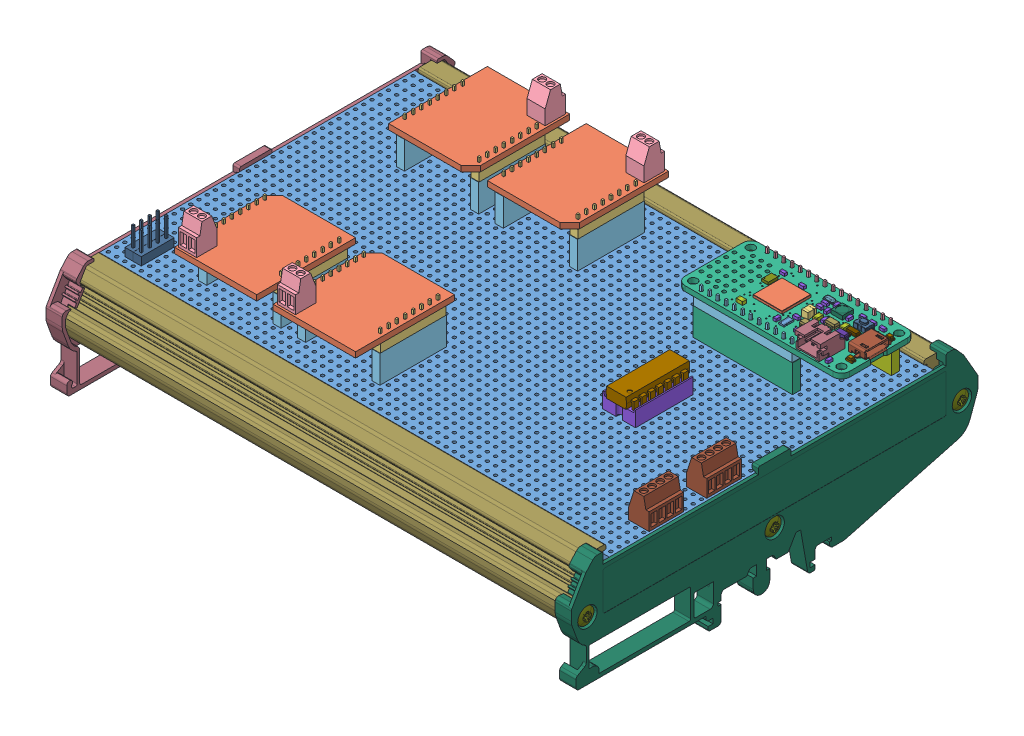
SolidWorks assembly custom_perfboard, configuration Default. Lengths in mm.
Overall size (162 55.7 125.4).
91 component instances, 34 part files, 27 mates.
Components (placement in the parent):
- perfboard-1: perfboard [Default] at origin size (160 1.6 100)
- 4-20mA_R_click_in_headers-1: 4-20mA_R_click_in_headers [Default] at (22.87 12.6 -69.05) size (25.4 24.5 30.48)
  - 4-20mA_R_click-1: 4-20mA_R_click [Default] at origin size (25.4 1.7 30.48)
  - header_m8-1: header_m8 [Default] at (1.25 -2.5 -22.86) x (0 0 1) z (-1 0 0) size (20.32 11.5 2.5)
  - header_m8-2: header_m8 [Default] at (24.15 -2.5 -2.54) x (0 0 -1) z (1 0 0) size (20.32 11.5 2.5)
  - screw_terminal_2x_2.54pitch-1: screw_terminal_2x_2.54pitch [Default] at (24.765 1.7 -23.545) x (0 0 -1) z (1 0 0) size (6.3 12.6 5.6)
  - header_f8-1: header_f8 [Default] at (24.15 -11 -2.415) x (0 0 -1) z (1 0 0) size (20.57 11.5 2.5)
  - header_f8-2: header_f8 [Default] at (1.25 -11 -22.985) x (0 0 1) z (-1 0 0) size (20.57 11.5 2.5)
- 4-20mA_R_click_in_headers-5: 4-20mA_R_click_in_headers [Default] at (48.27 12.6 -33.49) x (-1 0 0) z (0 0 -1) size (25.4 24.5 30.48)
  - 4-20mA_R_click-1: 4-20mA_R_click [Default] at origin size (25.4 1.7 30.48)
  - header_m8-1: header_m8 [Default] at (1.25 -2.5 -22.86) x (0 0 1) z (-1 0 0) size (20.32 11.5 2.5)
  - header_m8-2: header_m8 [Default] at (24.15 -2.5 -2.54) x (0 0 -1) z (1 0 0) size (20.32 11.5 2.5)
  - screw_terminal_2x_2.54pitch-1: screw_terminal_2x_2.54pitch [Default] at (24.765 1.7 -23.545) x (0 0 -1) z (1 0 0) size (6.3 12.6 5.6)
  - header_f8-1: header_f8 [Default] at (24.15 -11 -2.415) x (0 0 -1) z (1 0 0) size (20.57 11.5 2.5)
  - header_f8-2: header_f8 [Default] at (1.25 -11 -22.985) x (0 0 1) z (-1 0 0) size (20.57 11.5 2.5)
- 4-20mA_R_click_in_headers-2: 4-20mA_R_click_in_headers [Default] at (53.35 12.6 -69.05) size (25.4 24.5 30.48)
  - 4-20mA_R_click-1: 4-20mA_R_click [Default] at origin size (25.4 1.7 30.48)
  - header_m8-1: header_m8 [Default] at (1.25 -2.5 -22.86) x (0 0 1) z (-1 0 0) size (20.32 11.5 2.5)
  - header_m8-2: header_m8 [Default] at (24.15 -2.5 -2.54) x (0 0 -1) z (1 0 0) size (20.32 11.5 2.5)
  - screw_terminal_2x_2.54pitch-1: screw_terminal_2x_2.54pitch [Default] at (24.765 1.7 -23.545) x (0 0 -1) z (1 0 0) size (6.3 12.6 5.6)
  - header_f8-1: header_f8 [Default] at (24.15 -11 -2.415) x (0 0 -1) z (1 0 0) size (20.57 11.5 2.5)
  - header_f8-2: header_f8 [Default] at (1.25 -11 -22.985) x (0 0 1) z (-1 0 0) size (20.57 11.5 2.5)
- 3857 Adafruit Feather M4 Express headers 2-1: 3857 Adafruit Feather M4 Express headers 2 [Default] at (160.01 12.6 -94.45) x (-1 0 0) z (0 1 0) size (50.85 22.86 20.37)
  - 3857 Adafruit Feather M4 Express-1: 3857 Adafruit Feather M4 Express [Default] at origin size (50.85 22.86 6.37)
    - 3857 Adafruit Feather M4 Express(2)^3857 Adafruit Feather M4 Express-1: 3857 Adafruit Feather M4 Express(2)^3857 Adafruit Feather M4 Express [Default] at origin size (50.85 22.86 6.37) (virtual)
      - PCB Component^3857 Adafruit Feather M4 Express(2)_3857 Adafruit Feather M4 Express-1: PCB Component^3857 Adafruit Feather M4 Express(2)_3857 Adafruit Feather M4 Express [Default] at origin size (50.85 22.86 6.37) (virtual)
        - Board^PCB Component_3857 Adafruit Feather M4 Express(2)_3857 Adafruit Feather M4 Express-1: Board^PCB Component_3857 Adafruit Feather M4 Express(2)_3857 Adafruit Feather M4 Express [Default] at origin size (50.8 22.86 1.57) (virtual)
        - 10uF^PCB Component_3857 Adafruit Feather M4 Express(2)_3857 Adafruit Feather M4 Express-1: 10uF^PCB Component_3857 Adafruit Feather M4 Express(2)_3857 Adafruit Feather M4 Express [Default] at (12.042 9.838 1.57) x (0 -1 0) z (0 0 1) size (2 1.25 1) (virtual)
        - 10uF^PCB Component_3857 Adafruit Feather M4 Express(2)_3857 Adafruit Feather M4 Express-2: 10uF^PCB Component_3857 Adafruit Feather M4 Express(2)_3857 Adafruit Feather M4 Express [Default] at (14.728 13.858 1.57) size (2 1.25 1) (virtual)
        - 10uF^PCB Component_3857 Adafruit Feather M4 Express(2)_3857 Adafruit Feather M4 Express-3: 10uF^PCB Component_3857 Adafruit Feather M4 Express(2)_3857 Adafruit Feather M4 Express [Default] at (15.748 17.272 1.57) x (0 -1 0) z (0 0 1) size (2 1.25 1) (virtual)
        - 10uF^PCB Component_3857 Adafruit Feather M4 Express(2)_3857 Adafruit Feather M4 Express-4: 10uF^PCB Component_3857 Adafruit Feather M4 Express(2)_3857 Adafruit Feather M4 Express [Default] at (35.065 18.669 1.57) size (2 1.25 1) (virtual)
        - 10uF^PCB Component_3857 Adafruit Feather M4 Express(2)_3857 Adafruit Feather M4 Express-5: 10uF^PCB Component_3857 Adafruit Feather M4 Express(2)_3857 Adafruit Feather M4 Express [Default] at (18.796 11.303 1.57) x (0 -1 0) z (0 0 1) size (2 1.25 1) (virtual)
        - 1uF^PCB Component_3857 Adafruit Feather M4 Express(2)_3857 Adafruit Feather M4 Express-1: 1uF^PCB Component_3857 Adafruit Feather M4 Express(2)_3857 Adafruit Feather M4 Express [Default] at (24.909 17.78 1.57) x (0 1 0) z (0 0 1) size (1.6 0.9 0.8) (virtual)
        - 1uF^PCB Component_3857 Adafruit Feather M4 Express(2)_3857 Adafruit Feather M4 Express-2: 1uF^PCB Component_3857 Adafruit Feather M4 Express(2)_3857 Adafruit Feather M4 Express [Default] at (11.989 4.218 1.57) size (1.6 0.9 0.8) (virtual)
        - 1uF^PCB Component_3857 Adafruit Feather M4 Express(2)_3857 Adafruit Feather M4 Express-3: 1uF^PCB Component_3857 Adafruit Feather M4 Express(2)_3857 Adafruit Feather M4 Express [Default] at (5.715 20.955 1.57) x (0 -1 0) z (0 0 1) size (1.6 0.9 0.8) (virtual)
        - 1uF^PCB Component_3857 Adafruit Feather M4 Express(2)_3857 Adafruit Feather M4 Express-4: 1uF^PCB Component_3857 Adafruit Feather M4 Express(2)_3857 Adafruit Feather M4 Express [Default] at (5.829 4.254 1.57) size (1.6 0.9 0.8) (virtual)
        - 1uF^PCB Component_3857 Adafruit Feather M4 Express(2)_3857 Adafruit Feather M4 Express-5: 1uF^PCB Component_3857 Adafruit Feather M4 Express(2)_3857 Adafruit Feather M4 Express [Default] at (18.415 17.97 1.57) size (1.6 0.9 0.8) (virtual)
        - 1uF^PCB Component_3857 Adafruit Feather M4 Express(2)_3857 Adafruit Feather M4 Express-6: 1uF^PCB Component_3857 Adafruit Feather M4 Express(2)_3857 Adafruit Feather M4 Express [Default] at (19.202 5.067 1.57) x (0 1 0) z (0 0 1) size (1.6 0.9 0.8) (virtual)
        - 1uF^PCB Component_3857 Adafruit Feather M4 Express(2)_3857 Adafruit Feather M4 Express-7: 1uF^PCB Component_3857 Adafruit Feather M4 Express(2)_3857 Adafruit Feather M4 Express [Default] at (21.526 6.35 1.57) x (-1 0 0) z (0 0 1) size (1.6 0.9 0.8) (virtual)
        - 1uF^PCB Component_3857 Adafruit Feather M4 Express(2)_3857 Adafruit Feather M4 Express-8: 1uF^PCB Component_3857 Adafruit Feather M4 Express(2)_3857 Adafruit Feather M4 Express [Default] at (36.119 4.648 1.57) x (-1 0 0) z (0 0 1) size (1.6 0.9 0.8) (virtual)
        - 1uF^PCB Component_3857 Adafruit Feather M4 Express(2)_3857 Adafruit Feather M4 Express-9: 1uF^PCB Component_3857 Adafruit Feather M4 Express(2)_3857 Adafruit Feather M4 Express [Default] at (19.126 8.065 1.57) x (0 1 0) z (0 0 1) size (1.6 0.9 0.8) (virtual)
        - 1uF^PCB Component_3857 Adafruit Feather M4 Express(2)_3857 Adafruit Feather M4 Express-10: 1uF^PCB Component_3857 Adafruit Feather M4 Express(2)_3857 Adafruit Feather M4 Express [Default] at (29.662 5.263 1.57) x (-1 0 0) z (0 0 1) size (1.6 0.9 0.8) (virtual)
        - 1uF^PCB Component_3857 Adafruit Feather M4 Express(2)_3857 Adafruit Feather M4 Express-11: 1uF^PCB Component_3857 Adafruit Feather M4 Express(2)_3857 Adafruit Feather M4 Express [Default] at (8.89 4.254 1.57) x (-1 0 0) z (0 0 1) size (1.6 0.9 0.8) (virtual)
        - 1uF^PCB Component_3857 Adafruit Feather M4 Express(2)_3857 Adafruit Feather M4 Express-12: 1uF^PCB Component_3857 Adafruit Feather M4 Express(2)_3857 Adafruit Feather M4 Express [Default] at (17.145 10.922 1.57) x (0 1 0) z (0 0 1) size (1.6 0.9 0.8) (virtual)
        - 1uF^PCB Component_3857 Adafruit Feather M4 Express(2)_3857 Adafruit Feather M4 Express-13: 1uF^PCB Component_3857 Adafruit Feather M4 Express(2)_3857 Adafruit Feather M4 Express [Default] at (13.856 6.502 1.57) x (0 -1 0) z (0 0 1) size (1.6 0.9 0.8) (virtual)
        - 1uF^PCB Component_3857 Adafruit Feather M4 Express(2)_3857 Adafruit Feather M4 Express-14: 1uF^PCB Component_3857 Adafruit Feather M4 Express(2)_3857 Adafruit Feather M4 Express [Default] at (21.4 8.065 1.57) size (1.6 0.9 0.8) (virtual)
        - 1uF^PCB Component_3857 Adafruit Feather M4 Express(2)_3857 Adafruit Feather M4 Express-15: 1uF^PCB Component_3857 Adafruit Feather M4 Express(2)_3857 Adafruit Feather M4 Express [Default] at (22.225 14.414 1.57) x (-1 0 0) z (0 0 1) size (1.6 0.9 0.8) (virtual)
        - ORANGE^PCB Component_3857 Adafruit Feather M4 Express(2)_3857 Adafruit Feather M4 Express-1: ORANGE^PCB Component_3857 Adafruit Feather M4 Express(2)_3857 Adafruit Feather M4 Express [Default] at (2.645 17.359 1.57) x (0 1 0) z (0 0 1) size (1.25 2.02 1.1) (virtual)
        - ORANGE^PCB Component_3857 Adafruit Feather M4 Express(2)_3857 Adafruit Feather M4 Express-2: ORANGE^PCB Component_3857 Adafruit Feather M4 Express(2)_3857 Adafruit Feather M4 Express [Default] at (2.413 5.588 1.57) x (0 -1 0) z (0 0 1) size (1.25 2.02 1.1) (virtual)
        - KMR2^PCB Component_3857 Adafruit Feather M4 Express(2)_3857 Adafruit Feather M4 Express-1: KMR2^PCB Component_3857 Adafruit Feather M4 Express(2)_3857 Adafruit Feather M4 Express [Default] at (9.398 6.54 1.57) x (-1 0 0) z (0 0 1) size (4.6 2.8 1.94) (virtual)
        - microUSB^PCB Component_3857 Adafruit Feather M4 Express(2)_3857 Adafruit Feather M4 Express-1: microUSB^PCB Component_3857 Adafruit Feather M4 Express(2)_3857 Adafruit Feather M4 Express [Default] at (4.445 11.43 1.57) x (0 -1 0) z (0 0 1) size (8.8 5.6 3) (virtual)
        - MCP73831T-2ACI_OT^PCB Component_3857 Adafruit Feather M4 Express(2)_3857 Adafruit Feather M4 Express-1: MCP73831T-2ACI_OT^PCB Component_3857 Adafruit Feather M4 Express(2)_3857 Adafruit Feather M4 Express [Default] at (14.732 10.922 1.57) size (3 3 1.4) (virtual)
        - MCP73831T-2ACI_OT^PCB Component_3857 Adafruit Feather M4 Express(2)_3857 Adafruit Feather M4 Express-2: MCP73831T-2ACI_OT^PCB Component_3857 Adafruit Feather M4 Express(2)_3857 Adafruit Feather M4 Express [Default] at (18.352 15.113 1.57) size (3 3 1.4) (virtual)
        - JSTPH^PCB Component_3857 Adafruit Feather M4 Express(2)_3857 Adafruit Feather M4 Express-1: JSTPH^PCB Component_3857 Adafruit Feather M4 Express(2)_3857 Adafruit Feather M4 Express [Default] at (10.795 19.304 1.57) size (7.9 8.6 4.8) (virtual)
        - 32.768^PCB Component_3857 Adafruit Feather M4 Express(2)_3857 Adafruit Feather M4 Express-1: 32.768^PCB Component_3857 Adafruit Feather M4 Express(2)_3857 Adafruit Feather M4 Express [Default] at (21.806 4.496 1.57) x (-1 0 0) z (0 0 1) size (3.5 1.5 0.8) (virtual)
        - WS2812B3535^PCB Component_3857 Adafruit Feather M4 Express(2)_3857 Adafruit Feather M4 Express-1: WS2812B3535^PCB Component_3857 Adafruit Feather M4 Express(2)_3857 Adafruit Feather M4 Express [Default] at (16.485 6.109 1.57) x (0 -1 0) z (0 0 1) size (3.5 3.5 1.2) (virtual)
        - 2MB Flash^PCB Component_3857 Adafruit Feather M4 Express(2)_3857 Adafruit Feather M4 Express-1: 2MB Flash^PCB Component_3857 Adafruit Feather M4 Express(2)_3857 Adafruit Feather M4 Express [Default] at (36.512 8.433 1.57) x (0 1 0) z (0 0 1) size (3 2 0.8) (virtual)
        - MBR120^PCB Component_3857 Adafruit Feather M4 Express(2)_3857 Adafruit Feather M4 Express-1: MBR120^PCB Component_3857 Adafruit Feather M4 Express(2)_3857 Adafruit Feather M4 Express [Default] at (10.35 12.319 1.57) x (-1 0 0) z (0 0 1) size (3.6 1.4 1.35) (virtual)
        - DMG341^PCB Component_3857 Adafruit Feather M4 Express(2)_3857 Adafruit Feather M4 Express-1: DMG341^PCB Component_3857 Adafruit Feather M4 Express(2)_3857 Adafruit Feather M4 Express [Default] at (9.398 9.842 1.57) size (3.04 2.64 1.12) (virtual)
        - 100K^PCB Component_3857 Adafruit Feather M4 Express(2)_3857 Adafruit Feather M4 Express-1: 100K^PCB Component_3857 Adafruit Feather M4 Express(2)_3857 Adafruit Feather M4 Express [Default] at (22.67 17.208 1.57) x (0 1 0) z (0 0 1) size (3.05 1.6 0.5) (virtual)
        - ATSAMD51J^PCB Component_3857 Adafruit Feather M4 Express(2)_3857 Adafruit Feather M4 Express-1: ATSAMD51J^PCB Component_3857 Adafruit Feather M4 Express(2)_3857 Adafruit Feather M4 Express [Default] at (30.162 11.049 1.57) x (0 1 0) z (0 0 1) size (9 9 0.8) (virtual)
        - 10uH^PCB Component_3857 Adafruit Feather M4 Express(2)_3857 Adafruit Feather M4 Express-1: 10uH^PCB Component_3857 Adafruit Feather M4 Express(2)_3857 Adafruit Feather M4 Express [Default] at (21.082 11.811 1.57) x (0 -1 0) z (0 0 1) size (2.7 2 2) (virtual)
  - header_m16-1: header_m16 [Default] at (5.08 1.27 -2.5) x (1 0 0) z (0 -1 0) size (40.64 11.5 2.5)
  - header_m12-1: header_m12 [Default] at (15.24 21.59 -2.5) x (1 0 0) z (0 -1 0) size (30.48 11.5 2.5)
  - header_f12-1: header_f12 [Default] at (15.115 21.59 -11) x (1 0 0) z (0 -1 0) size (30.73 11.5 2.5)
  - header_f16-1: header_f16 [Default] at (4.955 1.27 -11) x (1 0 0) z (0 -1 0) size (40.89 11.5 2.5)
- dil_socket_2x7_populated-1: dil_socket_2x7_populated [Default] at (124.45 5.35 -38.57) x (0 0 -1) z (1 0 0) size (19.5 11.05 10.16)
  - dil_socket_2x7-1: dil_socket_2x7 [Default] at origin size (17.78 8.25 10.16)
  - dil_package_2x7-1: dil_package_2x7 [Default] at (-0.86 0.5 0) size (19.5 6.8 8.17)
- header_m4-1: header_m4 [Default] at (8.88 4.1 -15.71) x (0 0 1) z (1 0 0) size (10.16 11.5 2.5)
- header_m4-2: header_m4 [Default] at (6.34 4.1 -15.71) x (0 0 1) z (1 0 0) size (10.16 11.5 2.5)
- screw_terminal_4x_2.54pitch_Multicomp_MP008515-1: screw_terminal_4x_2.54pitch_Multicomp_MP008515 [Default] at (153.05 1.6 -12.93) size (6.3 12.4 10.64)
- screw_terminal_4x_2.54pitch_Multicomp_MP008515-2: screw_terminal_4x_2.54pitch_Multicomp_MP008515 [Default] at (153.05 1.6 -30.71) size (6.3 12.4 10.64)
- 4-20mA_R_click_in_headers-6: 4-20mA_R_click_in_headers [Default] at (78.75 12.6 -33.49) x (-1 0 0) z (0 0 -1) size (25.4 24.5 30.48)
  - 4-20mA_R_click-1: 4-20mA_R_click [Default] at origin size (25.4 1.7 30.48)
  - header_m8-1: header_m8 [Default] at (1.25 -2.5 -22.86) x (0 0 1) z (-1 0 0) size (20.32 11.5 2.5)
  - header_m8-2: header_m8 [Default] at (24.15 -2.5 -2.54) x (0 0 -1) z (1 0 0) size (20.32 11.5 2.5)
  - screw_terminal_2x_2.54pitch-1: screw_terminal_2x_2.54pitch [Default] at (24.765 1.7 -23.545) x (0 0 -1) z (1 0 0) size (6.3 12.6 5.6)
  - header_f8-1: header_f8 [Default] at (24.15 -11 -2.415) x (0 0 -1) z (1 0 0) size (20.57 11.5 2.5)
  - header_f8-2: header_f8 [Default] at (1.25 -11 -22.985) x (0 0 1) z (-1 0 0) size (20.57 11.5 2.5)
- Damen_CNC_2340-1_DIN-Rail_Mount_for_Eurocard_PCB_100x160mm_STEP214-1: Damen_CNC_2340-1_DIN-Rail_Mount_for_Eurocard_PCB_100x160mm_STEP214 [Default] at (158 -16.0731 10.0976) x (0 1 0) z (-1 0 0) size (37.6 125.4 162)
  - 2340-1_DIN-Rail_Mount_for_Eurocard_PCB_100x160mm_STEP214^Damen_CNC_2340-1_DIN-Rail_Mount_for_Eurocard_PCB_100x160mm_STEP214-1: 2340-1_DIN-Rail_Mount_for_Eurocard_PCB_100x160mm_STEP214^Damen_CNC_2340-1_DIN-Rail_Mount_for_Eurocard_PCB_100x160mm_STEP214 [Default] at origin size (37.6 125.4 162) (virtual)
    - eBom-prt0^2340-1_DIN-Rail_Mount_for_Eurocard_PCB_100x160mm_STEP214_Damen_CNC_2340-1_DIN-Rail_Mount_for_Eurocard_PCB_100x160mm_STEP214-1: eBom-prt0^2340-1_DIN-Rail_Mount_for_Eurocard_PCB_100x160mm_STEP214_Damen_CNC_2340-1_DIN-Rail_Mount_for_Eurocard_PCB_100x160mm_STEP214 [Default] at (-0.1593 -0.1673 0) size (21.5 122.6 156) (virtual)
    - eBom-prt1^2340-1_DIN-Rail_Mount_for_Eurocard_PCB_100x160mm_STEP214_Damen_CNC_2340-1_DIN-Rail_Mount_for_Eurocard_PCB_100x160mm_STEP214-1: eBom-prt1^2340-1_DIN-Rail_Mount_for_Eurocard_PCB_100x160mm_STEP214_Damen_CNC_2340-1_DIN-Rail_Mount_for_Eurocard_PCB_100x160mm_STEP214 [Default] at (-4.4655 32.2694 159) x (0 1 0) z (0 0 1) size (125.4 37.6 5) (virtual)
    - eBom-prt2^2340-1_DIN-Rail_Mount_for_Eurocard_PCB_100x160mm_STEP214_Damen_CNC_2340-1_DIN-Rail_Mount_for_Eurocard_PCB_100x160mm_STEP214-1: eBom-prt2^2340-1_DIN-Rail_Mount_for_Eurocard_PCB_100x160mm_STEP214_Damen_CNC_2340-1_DIN-Rail_Mount_for_Eurocard_PCB_100x160mm_STEP214 [Default] at (14.3514 121.3074 83.05) x (0.707107 -0.707107 0) z (0 0 1) size (5.4 5.4 15.85) (virtual)
    - eBom-prt2^2340-1_DIN-Rail_Mount_for_Eurocard_PCB_100x160mm_STEP214_Damen_CNC_2340-1_DIN-Rail_Mount_for_Eurocard_PCB_100x160mm_STEP214-2: eBom-prt2^2340-1_DIN-Rail_Mount_for_Eurocard_PCB_100x160mm_STEP214_Damen_CNC_2340-1_DIN-Rail_Mount_for_Eurocard_PCB_100x160mm_STEP214 [Default] at (9.3514 63.5574 83.05) x (0.707107 -0.707107 0) z (0 0 1) size (5.4 5.4 15.85) (virtual)
    - eBom-prt2^2340-1_DIN-Rail_Mount_for_Eurocard_PCB_100x160mm_STEP214_Damen_CNC_2340-1_DIN-Rail_Mount_for_Eurocard_PCB_100x160mm_STEP214-3: eBom-prt2^2340-1_DIN-Rail_Mount_for_Eurocard_PCB_100x160mm_STEP214_Damen_CNC_2340-1_DIN-Rail_Mount_for_Eurocard_PCB_100x160mm_STEP214 [Default] at (14.3514 5.8074 83.05) x (0.707107 -0.707107 0) z (0 0 1) size (5.4 5.4 15.85) (virtual)
    - eBom-prt3^2340-1_DIN-Rail_Mount_for_Eurocard_PCB_100x160mm_STEP214_Damen_CNC_2340-1_DIN-Rail_Mount_for_Eurocard_PCB_100x160mm_STEP214-1: eBom-prt3^2340-1_DIN-Rail_Mount_for_Eurocard_PCB_100x160mm_STEP214_Damen_CNC_2340-1_DIN-Rail_Mount_for_Eurocard_PCB_100x160mm_STEP214 [Default] at (-11.9191 -27.5171 -9.3242) x (0 1 0) z (0 0 -1) size (125.4 37.6 5) (virtual)
    - eBom-prt4^2340-1_DIN-Rail_Mount_for_Eurocard_PCB_100x160mm_STEP214_Damen_CNC_2340-1_DIN-Rail_Mount_for_Eurocard_PCB_100x160mm_STEP214-1: eBom-prt4^2340-1_DIN-Rail_Mount_for_Eurocard_PCB_100x160mm_STEP214_Damen_CNC_2340-1_DIN-Rail_Mount_for_Eurocard_PCB_100x160mm_STEP214 [Default] at (14.3514 114.3878 70.95) x (0.707107 0.707107 0) z (0 0 -1) size (5.15 5.15 16) (virtual)
    - eBom-prt4^2340-1_DIN-Rail_Mount_for_Eurocard_PCB_100x160mm_STEP214_Damen_CNC_2340-1_DIN-Rail_Mount_for_Eurocard_PCB_100x160mm_STEP214-2: eBom-prt4^2340-1_DIN-Rail_Mount_for_Eurocard_PCB_100x160mm_STEP214_Damen_CNC_2340-1_DIN-Rail_Mount_for_Eurocard_PCB_100x160mm_STEP214 [Default] at (-7.2051 63.5574 70.95) x (-0.707107 -0.707107 0) z (0 0 -1) size (5.15 5.15 16) (virtual)
    - eBom-prt4^2340-1_DIN-Rail_Mount_for_Eurocard_PCB_100x160mm_STEP214_Damen_CNC_2340-1_DIN-Rail_Mount_for_Eurocard_PCB_100x160mm_STEP214-3: eBom-prt4^2340-1_DIN-Rail_Mount_for_Eurocard_PCB_100x160mm_STEP214_Damen_CNC_2340-1_DIN-Rail_Mount_for_Eurocard_PCB_100x160mm_STEP214 [Default] at (-2.2051 5.8074 70.95) x (-0.707107 -0.707107 0) z (0 0 -1) size (5.15 5.15 16) (virtual)
Mates (geometry in assembly coordinates):
- Concentric1: concentric aligned: line of 4-20mA_R_click_in_headers-1/header_f8-2 through (24.12 1.6 -90.64) axis (0 -1 0); cylinder of perfboard-1 through (24.12 1.601 -90.64) axis (0 -1 0) radius 0.5
- Coincident1: coincident anti-aligned: plane of perfboard-1 through (0 1.6 0) normal (0 1 0); plane of 4-20mA_R_click_in_headers-1/header_f8-2 through (22.87 1.6 -92.035) normal (0 -1 0)
- Parallel1: parallel aligned: plane of 4-20mA_R_click_in_headers-1 through (22.87 12.6 -69.05) normal (1 0 0)
- Coincident3: coincident anti-aligned: plane of perfboard-1 through (0 1.6 0) normal (0 1 0); plane of 3857 Adafruit Feather M4 Express headers 2-1/header_f12-1 through (144.895 1.6 -74.11) normal (0 -1 0)
- Parallel2: parallel aligned: plane of 3857 Adafruit Feather M4 Express headers 2-1/3857 Adafruit Feather M4 Express-1/3857 Adafruit Feather M4 Express(2)^3857 Adafruit Feather M4 Express-1/PCB Component^3857 Adafruit Feather M4 Express(2)_3857 Adafruit Feather M4 Express-1/Board^PCB Component_3857 Adafruit Feather M4 Express(2)_3857 Adafruit Feather M4 Express-1 through (160.01 12.6 -94.45) normal (0 0 1); plane of assembly through (0 0 0) normal (0 0 1)
- Concentric3: concentric aligned: line of 3857 Adafruit Feather M4 Express headers 2-1/header_f12-1 through (143.5 1.6 -72.86) axis (0 -1 0); cylinder of perfboard-1 through (143.5 1.601 -72.86) axis (0 -1 0) radius 0.5
- Coincident5: coincident anti-aligned: plane of perfboard-1 through (0 1.6 0) normal (0 1 0); plane of dil_socket_2x7_populated-1/dil_socket_2x7-1 through (129.53 1.6 -56.35) normal (0 -1 0)
- Parallel3: parallel aligned: plane of dil_socket_2x7_populated-1 through (124.45 5.35 -38.57) normal (1 0 0)
- Concentric4: concentric aligned: line of dil_socket_2x7_populated-1/dil_socket_2x7-1 through (128.26 10.1661 -39.84) axis (0 -1 0); cylinder of perfboard-1 through (128.26 1.601 -39.84) axis (0 -1 0) radius 0.5
- Coincident8: coincident anti-aligned: plane of perfboard-1 through (0 1.6 0) normal (0 1 0); plane of header_m4-1 through (10.13 1.6 -15.71) normal (0 -1 0)
- Coincident10: coincident anti-aligned: plane of perfboard-1 through (0 1.6 0) normal (0 1 0); plane of header_m4-2 through (7.59 1.6 -15.71) normal (0 -1 0)
- Parallel5: parallel aligned: plane of header_m4-1 through (8.88 4.1 -15.71) normal (1 0 0)
- Concentric6: concentric anti-aligned: line of header_m4-1 through (8.88 4.1 -14.44) axis (0 1 0); cylinder of perfboard-1 through (8.88 1.601 -14.44) axis (0 -1 0) radius 0.5
- Coincident15: coincident aligned: plane of header_m4-1 through (8.88 4.1 -15.71) normal (0 0 1); plane of header_m4-2 through (6.34 4.1 -15.71) normal (0 0 1)
- Distance1: distance = 2.54 mm aligned: plane of header_m4-2 through (6.34 4.1 -15.71) normal (1 0 0); plane of header_m4-1 through (8.88 4.1 -15.71) normal (1 0 0)
- Coincident17: coincident anti-aligned: plane of perfboard-1 through (0 1.6 0) normal (0 1 0); plane of 4-20mA_R_click_in_headers-5/header_f8-1 through (22.87 1.6 -31.075) normal (0 -1 0)
- Coincident18: coincident aligned: plane of 4-20mA_R_click_in_headers-1/header_f8-2 through (22.87 1.6 -92.035) normal (-1 0 0); plane of 4-20mA_R_click_in_headers-5/header_f8-1 through (22.87 1.6 -31.075) normal (-1 0 0)
- Concentric9: concentric aligned: cylinder of perfboard-1 through (24.12 1.601 -11.9) axis (0 -1 0) radius 0.5; line of 4-20mA_R_click_in_headers-5/header_f8-1 through (24.12 1.6 -11.9) axis (0 -1 0)
- Coincident19: coincident aligned: plane of perfboard-1 through (80 0 0) normal (1 0 0); plane of Damen_CNC_2340-1_DIN-Rail_Mount_for_Eurocard_PCB_100x160mm_STEP214-1 through (80 -16.0731 10.0976) normal (1 0 0)
- Coincident20: coincident aligned: plane of perfboard-1 through (0 0 -50) normal (0 0 1); plane of Damen_CNC_2340-1_DIN-Rail_Mount_for_Eurocard_PCB_100x160mm_STEP214-1 through (158 -16.0731 -50) normal (0 0 1)
- Coincident21: coincident anti-aligned: plane of perfboard-1 through (0 0 0) normal (0 -1 0); plane of Damen_CNC_2340-1_DIN-Rail_Mount_for_Eurocard_PCB_100x160mm_STEP214-1 through (158 0 10.0976) normal (0 1 0)
- Coincident22: coincident anti-aligned: plane of perfboard-1 through (0 1.6 0) normal (0 1 0); plane of screw_terminal_4x_2.54pitch_Multicomp_MP008515-2 through (159.35 1.6 -41.35) normal (0 -1 0)
- Coincident23: coincident anti-aligned: plane of perfboard-1 through (0 1.6 0) normal (0 1 0); plane of screw_terminal_4x_2.54pitch_Multicomp_MP008515-1 through (159.35 1.6 -23.57) normal (0 -1 0)
- Parallel6: parallel aligned: plane of screw_terminal_4x_2.54pitch_Multicomp_MP008515-1 through (153.05 1.6 -12.93) normal (1 0 0)
- Parallel7: parallel aligned: plane of screw_terminal_4x_2.54pitch_Multicomp_MP008515-2 through (153.05 1.6 -30.71) normal (1 0 0)
- Concentric10: concentric aligned: line of screw_terminal_4x_2.54pitch_Multicomp_MP008515-1 through (156.2 1.6 -14.44) axis (0 -1 0); cylinder of perfboard-1 through (156.2 1.601 -14.44) axis (0 -1 0) radius 0.5
- Concentric11: concentric aligned: line of screw_terminal_4x_2.54pitch_Multicomp_MP008515-2 through (156.2 1.6 -32.22) axis (0 -1 0); cylinder of perfboard-1 through (156.2 1.601 -32.22) axis (0 -1 0) radius 0.5
